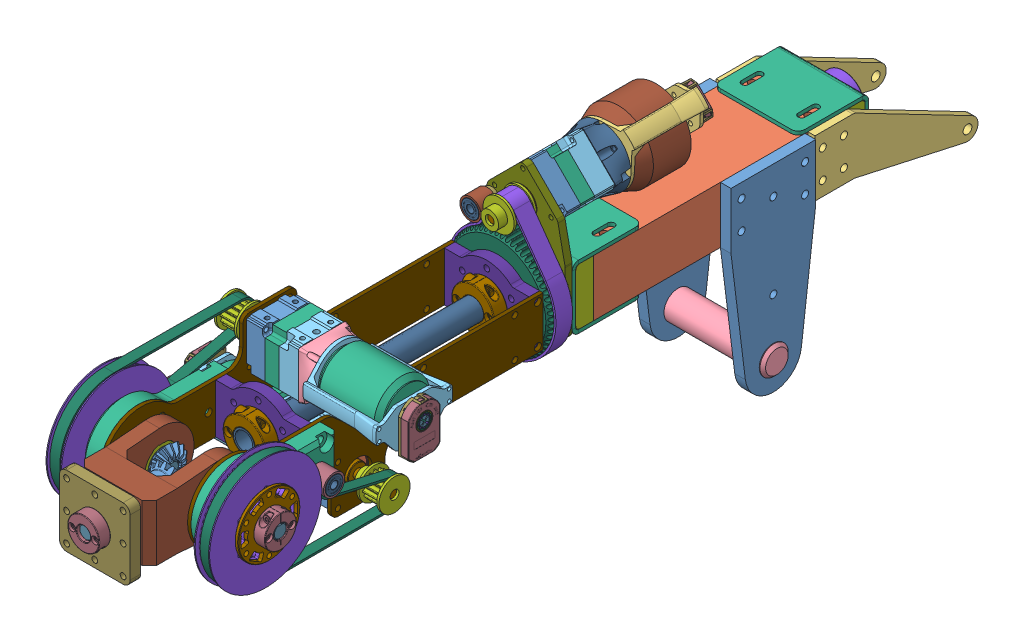
SolidWorks assembly Forearm, configuration Default. Lengths in mm. (continued)
Components (placement in the parent): (continued)
- 15Tpulley-4: 15Tpulley [Default] at (0 823.07 189.5517) x (-0.382318 -0.924031 0) z (-0.924031 0.382318 0) size (28 28 28)
- 15Tpulley-5: 15Tpulley [Default] at (-64.1092 796.898 367.2673) x (0 -1 0) z (0 0 1) size (28 28 28)
- 15Tpulley-6: 15Tpulley [Default] at (64.1092 726.052 367.2673) x (0 1 0) z (0 0 1) size (28 28 28)
- J4Belt^Forearm-1: J4Belt^Forearm [Default] at origin size (97.23 123.02 15) (virtual)
- TensionPillarJ4-1: TensionPillarJ4 [Default] at (30.7519 716.5034 107.0507) x (-0.923728 -0.383049 0) z (0.383049 -0.923728 0) size (19.05 19.38 19.05)
  - 98019A228_MIL SPEC. 300 SERIES SS FLAT WASHER-1: 98019A228_MIL SPEC. 300 SERIES SS FLAT WASHER [98019A228] at (17.4581 -74.6355 -111.1226) x (0.972939 0 -0.231063) z (0.231063 0 0.972939) size (9.53 0.71 9.53)
  - 60355K701_BALL BEARING-1: 60355K701_BALL BEARING [60355K701] at (17.4581 -77.1247 -111.1226) x (1 0 0) z (0 1 0) size (15.88 15.88 4.98)
  - Roller^TensionPillarJ4-1: Roller^TensionPillarJ4 [Default] at (-4.9135 -16.9545 2.0107) size (19.05 15 19.05) (virtual)
  - 60355K701_BALL BEARING-2: 60355K701_BALL BEARING [60355K701] at (17.4581 -87.6441 -111.1226) x (1 0 0) z (0 1 0) size (15.88 15.88 4.98)
  - 92510A483_ALUM UNTHRD SPACER-1: 92510A483_ALUM UNTHRD SPACER [92510A483] at (17.4581 -72.3368 -111.1226) x (1 0 0) z (0 1 0) size (15.88 15.88 3.17)
- TensionPillarJ56-1: TensionPillarJ56 [Default] at (15.1868 665.5152 480.9669) x (0 -0.383049 -0.923728) z (0 -0.923728 0.383049) size (19.05 17.8 19.05)
  - 98019A228_MIL SPEC. 300 SERIES SS FLAT WASHER-1: 98019A228_MIL SPEC. 300 SERIES SS FLAT WASHER [98019A228] at (17.4581 -74.6355 -111.1226) x (0.972939 0 -0.231063) z (0.231063 0 0.972939) size (9.53 0.71 9.53)
  - 60355K701_BALL BEARING-1: 60355K701_BALL BEARING [60355K701] at (17.4581 -77.1247 -111.1226) x (1 0 0) z (0 1 0) size (15.88 15.88 4.98)
  - Roller^TensionPillarJ56-1: Roller^TensionPillarJ56 [Default] at (-4.9135 -16.9545 2.0107) size (19.05 15 19.05) (virtual)
  - 60355K701_BALL BEARING-2: 60355K701_BALL BEARING [60355K701] at (17.4581 -87.6441 -111.1226) x (1 0 0) z (0 1 0) size (15.88 15.88 4.98)
  - 92510A398_ALUM UNTHRD SPACER-1: 92510A398_ALUM UNTHRD SPACER [92510A398] at (17.4581 -73.1305 -111.1226) x (1 0 0) z (0 1 0) size (12.7 12.7 1.59)
- J56Belt^Forearm-1: J56Belt^Forearm [Default] at origin size (9 97.23 176.76) (virtual)
- TensionPillarJ56-2: TensionPillarJ56 [Default] at (-15.1868 870.8093 395.8361) x (0 -0.383049 -0.923728) z (0 0.923728 -0.383049) size (19.05 17.8 19.05)
  - 98019A228_MIL SPEC. 300 SERIES SS FLAT WASHER-1: 98019A228_MIL SPEC. 300 SERIES SS FLAT WASHER [98019A228] at (17.4581 -74.6355 -111.1226) x (0.972939 0 -0.231063) z (0.231063 0 0.972939) size (9.53 0.71 9.53)
  - 60355K701_BALL BEARING-1: 60355K701_BALL BEARING [60355K701] at (17.4581 -77.1247 -111.1226) x (1 0 0) z (0 1 0) size (15.88 15.88 4.98)
  - Roller^TensionPillarJ56-1: Roller^TensionPillarJ56 [Default] at (-4.9135 -16.9545 2.0107) size (19.05 15 19.05) (virtual)
  - 60355K701_BALL BEARING-2: 60355K701_BALL BEARING [60355K701] at (17.4581 -87.6441 -111.1226) x (1 0 0) z (0 1 0) size (15.88 15.88 4.98)
  - 92510A398_ALUM UNTHRD SPACER-1: 92510A398_ALUM UNTHRD SPACER [92510A398] at (17.4581 -73.1305 -111.1226) x (1 0 0) z (0 1 0) size (12.7 12.7 1.59)
- J56Belt^Forearm-2: J56Belt^Forearm [Default] at (0 1522.95 0) x (-1 0 0) z (0 0 1) size (9 97.23 176.76) (virtual)
Mates (geometry in assembly coordinates):
- Concentric1: concentric anti-aligned: cylinder of SidePlate^Forearm-1 through (-47.625 634.475 0) axis (1 0 0) radius 12.7; circle of 6061K602_HARDENED PRECISION STEEL SHAFT-1
- Width1: width anti-aligned: plane of 6061K602_HARDENED PRECISION STEEL SHAFT-1 through (-50.8 634.475 0) normal (-1 0 0); plane of 6061K602_HARDENED PRECISION STEEL SHAFT-1 through (50.8 634.475 0) normal (1 0 0); plane of SidePlate^Forearm-2 through (47.625 634.475 0) normal (1 0 0); plane of SidePlate^Forearm-1 through (-47.625 634.475 0) normal (-1 0 0)
- Concentric2: concentric aligned: cylinder of 6384K367_BALL BEARING-1 through (0 761.475 160.274) axis (0 0 -1) radius 20.6375; cylinder of BearingHolder^Forearm-1 through (0 761.475 171.45) axis (0 0 -1) radius 20.6375
- Coincident2: coincident anti-aligned: plane of 6384K367_BALL BEARING-1 through (0 746.0646 171.45) normal (0 0 -1); plane of BearingHolder^Forearm-1 through (0 0 171.45) normal (0 0 1)
- Concentric3: concentric aligned: cylinder of 6384K367_BALL BEARING-2 through (0 761.475 -84.074) axis (0 0 1) radius 9.525; cylinder of 6435K160_ONE-PIECE CLAMP-ON SHAFT COLLAR-1 through (0 761.475 -111.0742) axis (0 0 1) radius 9.525
- Coincident3: coincident anti-aligned: plane of 6384K367_BALL BEARING-2 through (0 750.6038 -98.3742) normal (0 0 -1); plane of 6435K160_ONE-PIECE CLAMP-ON SHAFT COLLAR-1 through (0 761.475 -98.3742) normal (0 0 1)
- Concentric4: concentric anti-aligned: cylinder of 6384K367_BALL BEARING-1 through (0 761.475 160.274) axis (0 0 -1) radius 9.525; cylinder of 9677T100_CLAMP-ON SHAFT COLLAR WITH MOUNTING HOLES-1 through (0 761.475 210.2517) axis (0 0 1) radius 9.525
- Concentric5: concentric anti-aligned: cylinder of 89955K599_Tube^Forearm-1 through (0 761.475 455.5658) axis (0 0 -1) radius 9.525; cylinder of 5909K460_THRUST NEEDLE-ROLLER BEARING-1 through (0 761.475 187.5917) axis (0 0 1) radius 9.5504
- Coincident4: coincident anti-aligned: plane of ThrustBase^Forearm-1 through (0 761.475 187.5917) normal (0 0 1); plane of 5909K460_THRUST NEEDLE-ROLLER BEARING-1 through (0 761.475 187.5917) normal (0 0 -1)
- Concentric6: concentric anti-aligned: cylinder of 89955K599_Tube^Forearm-1 through (0 761.475 455.5658) axis (0 0 -1) radius 9.525; cylinder of 5909K330_THRUST NEEDLE-ROLLER BEARING-1 through (0 761.475 190.3889) axis (0 0 1) radius 9.5504
- Tangent1: tangent anti-aligned: plane of 5909K460_THRUST NEEDLE-ROLLER BEARING-1 through (0 761.475 188.4045) normal (0 0 1); cylinder of 5909K330_THRUST NEEDLE-ROLLER BEARING-1 through (-5.4469 747.7178 189.3967) axis (-0.368125 -0.929776 0) radius 0.9922
- Concentric7: concentric anti-aligned: cylinder of 89955K599_Tube^Forearm-1 through (0 761.475 455.5658) axis (0 0 -1) radius 9.525; cylinder of 5909K460_THRUST NEEDLE-ROLLER BEARING-2 through (0 761.475 190.3889) axis (0 0 1) radius 9.5504
- Tangent2: tangent anti-aligned: cylinder of 5909K330_THRUST NEEDLE-ROLLER BEARING-1 through (-1.8545 746.7954 189.3967) axis (-0.125333 -0.992115 0) radius 0.9922; plane of 5909K460_THRUST NEEDLE-ROLLER BEARING-2 through (0 761.475 190.3889) normal (0 0 -1)
- Concentric8: concentric anti-aligned: cylinder of 89955K599_Tube^Forearm-1 through (0 761.475 455.5658) axis (0 0 -1) radius 9.525; circle of J4Pulley-1
- Coincident6: coincident anti-aligned: plane of PulleySupportPlate^Forearm-1 through (0 0 194.3767) normal (0 0 1); plane of J4Pulley-1 through (0 761.475 194.3767) normal (0 0 -1)
- Parallel1: parallel anti-aligned: plane of 9677T100_CLAMP-ON SHAFT COLLAR WITH MOUNTING HOLES-1 through (0.0953 780.5248 210.2517) normal (-1 0 0)
- Coincident11: coincident anti-aligned: plane of 9677T100_CLAMP-ON SHAFT COLLAR WITH MOUNTING HOLES-1 through (0 761.475 210.2517) normal (0 0 -1); plane of WristHub^Forearm-1 through (-24.5934 788.4625 210.2517) normal (0 0 1)
- Concentric10: concentric aligned: cylinder of 89955K599_Tube^Forearm-1 through (0 761.475 455.5658) axis (0 0 -1) radius 9.525; cylinder of WristHub^Forearm-2 through (0 761.475 415.925) axis (0 0 -1) radius 9.525
- Distance2: distance = 406.4 mm: plane of assembly through (0 0 0) normal (0 0 1); plane of assembly; plane of WristHub^Forearm-2 through (-24.5934 788.4625 406.4) normal (0 0 -1)
- Concentric11: concentric anti-aligned: cylinder of 89955K599_Tube^Forearm-1 through (0 761.475 455.5658) axis (0 0 -1) radius 7.9375; cylinder of 9677T100_CLAMP-ON SHAFT COLLAR WITH MOUNTING HOLES-2 through (0 761.475 415.925) axis (0 0 1) radius 9.525
- Coincident13: coincident anti-aligned: plane of WristHub^Forearm-2 through (-24.5934 788.4625 415.925) normal (0 0 1); plane of 9677T100_CLAMP-ON SHAFT COLLAR WITH MOUNTING HOLES-2 through (0 761.475 415.925) normal (0 0 -1)
- Concentric12: concentric anti-aligned: cylinder of WristSidePlate^Forearm-1 through (-41.275 761.475 482.6) axis (1 0 0) radius 14.2875; cylinder of 6843K130_MTL MITER GEAR--20 DEG PRESSURE ANGLE-1 through (31.0355 761.475 482.6) axis (-1 0 0) radius 6.3563
- Concentric13: concentric anti-aligned: cylinder of 89955K599_Tube^Forearm-1 through (0 761.475 455.5658) axis (0 0 -1) radius 7.9375; cylinder of 6843K130_MTL MITER GEAR--20 DEG PRESSURE ANGLE-3 through (0 761.475 451.5645) axis (0 0 1) radius 6.3563
- Distance3: distance = 31.75 mm: cylinder of 6843K130_MTL MITER GEAR--20 DEG PRESSURE ANGLE-3 through (0 761.475 451.5645) axis (0 0 1) radius 6.3563; plane of 6843K130_MTL MITER GEAR--20 DEG PRESSURE ANGLE-1 through (-31.75 761.253 469.9019) normal (-1 0 0)
- Distance4: distance = 31.75 mm: plane of 6843K130_MTL MITER GEAR--20 DEG PRESSURE ANGLE-3 through (-12.6981 761.253 514.35) normal (0 0 1); cylinder of 6843K130_MTL MITER GEAR--20 DEG PRESSURE ANGLE-1 through (31.0355 761.475 482.6) axis (-1 0 0) radius 6.3563
- Concentric14: concentric anti-aligned: cylinder of WristSidePlate^Forearm-1 through (-41.275 761.475 482.6) axis (1 0 0) radius 14.2875; cylinder of 6384K361_BALL BEARING-1-1 through (-46.101 761.475 482.6) axis (-1 0 0) radius 14.2875
- Coincident14: coincident anti-aligned: plane of WristSidePlate^Forearm-1 through (-38.1 0 0) normal (1 0 0); plane of 6384K361_BALL BEARING-1-1 through (-38.1 772.1938 482.6) normal (-1 0 0)
- Concentric15: concentric aligned: cylinder of 6843K130_MTL MITER GEAR--20 DEG PRESSURE ANGLE-1 through (31.0355 761.475 482.6) axis (-1 0 0) radius 6.3563; cylinder of 5909K440_THRUST NEEDLE-ROLLER BEARING-1 through (-33.7344 761.475 482.6) axis (-1 0 0) radius 6.3754
- Concentric16: concentric anti-aligned: cylinder of 6843K130_MTL MITER GEAR--20 DEG PRESSURE ANGLE-1 through (31.0355 761.475 482.6) axis (-1 0 0) radius 6.3563; cylinder of 5909K310_THRUST NEEDLE-ROLLER BEARING-1 through (-31.75 761.475 482.6) axis (1 0 0) radius 6.3754
- Tangent6: tangent anti-aligned: plane of 6843K130_MTL MITER GEAR--20 DEG PRESSURE ANGLE-1 through (-31.75 761.253 469.9019) normal (-1 0 0); cylinder of 5909K310_THRUST NEEDLE-ROLLER BEARING-1 through (-32.7422 750.594 485.3554) axis (0 -0.9694 0.245485) radius 0.9922
- Tangent7: tangent anti-aligned: plane of 5909K440_THRUST NEEDLE-ROLLER BEARING-1 through (-33.7344 761.475 482.6) normal (1 0 0); cylinder of 5909K310_THRUST NEEDLE-ROLLER BEARING-1 through (-32.7422 750.594 485.3554) axis (0 -0.9694 0.245485) radius 0.9922
- Concentric17: concentric aligned: cylinder of 6384K361_BALL BEARING-1-2 through (-49.149 761.475 482.6) axis (1 0 0) radius 14.2875; cylinder of SidePrintedSupport^Forearm-1 through (-57.15 761.475 482.6) axis (1 0 0) radius 14.2875
- Coincident16: coincident anti-aligned: plane of SidePrintedSupport^Forearm-1 through (-57.15 0 0) normal (-1 0 0); plane of 6384K361_BALL BEARING-1-2 through (-57.15 750.7562 482.6) normal (1 0 0)
- Concentric18: concentric anti-aligned: cylinder of 6843K130_MTL MITER GEAR--20 DEG PRESSURE ANGLE-1 through (31.0355 761.475 482.6) axis (-1 0 0) radius 12.7; cylinder of 6391K281_OIL-EMBEDDED SLEEVE BEARING-1 through (-32.2445 761.475 482.6) axis (1 0 0) radius 12.7
- Concentric20: concentric anti-aligned: cylinder of 6384K361_BALL BEARING-1-2 through (-49.149 761.475 482.6) axis (1 0 0) radius 6.35; cylinder of PulleyHubbed-1/1_2_ID_1_8_Keyway_Aluminum_VersaHub_217-2590 v1-1 through (-64.0842 761.475 482.6) axis (-1 0 0) radius 6.3627
- Coincident18: coincident anti-aligned: plane of PulleyHubbed-1/1_2_ID_1_8_Keyway_Aluminum_VersaHub_217-2590 v1-1 through (-64.0842 761.475 482.6) normal (1 0 0); plane of SidePulleySpacer^Forearm-1 through (-64.0842 761.475 482.6) normal (-1 0 0)
- Concentric21: concentric anti-aligned: cylinder of WristBase^Forearm-3 through (0 761.475 546.1) axis (0 0 -1) radius 14.2875; cylinder of 6384K361_BALL BEARING-1-5 through (0 761.475 528.701) axis (0 0 1) radius 14.2875
- Coincident19: coincident anti-aligned: plane of WristBase^Forearm-3 through (0 0 520.7) normal (0 0 -1); plane of 6384K361_BALL BEARING-1-5 through (0 772.1938 520.7) normal (0 0 1)
- Concentric22: concentric anti-aligned: cylinder of WristBase^Forearm-3 through (0 761.475 546.1) axis (0 0 -1) radius 14.2875; cylinder of MiterSpacer^Forearm-3 through (0 761.475 472.2459) axis (0 0 1) radius 9.3726
- Coincident21: coincident anti-aligned: plane of 6384K361_BALL BEARING-1-5 through (0 775.2862 519.176) normal (0 0 -1); plane of MiterSpacer^Forearm-3 through (0 761.475 519.176) normal (0 0 1)
- Concentric23: concentric anti-aligned: cylinder of WristBase^Forearm-3 through (0 761.475 546.1) axis (0 0 -1) radius 14.2875; cylinder of 5909K440_THRUST NEEDLE-ROLLER BEARING-3 through (0 761.475 516.3344) axis (0 0 1) radius 6.3754
- Coincident22: coincident anti-aligned: plane of MiterSpacer^Forearm-3 through (0 761.475 517.1472) normal (0 0 -1); plane of 5909K440_THRUST NEEDLE-ROLLER BEARING-3 through (0 761.475 517.1472) normal (0 0 1)
- Concentric24: concentric anti-aligned: cylinder of WristBase^Forearm-3 through (0 761.475 546.1) axis (0 0 -1) radius 14.2875; cylinder of 5909K310_THRUST NEEDLE-ROLLER BEARING-3 through (0 761.475 516.3344) axis (0 0 1) radius 6.3754
- Tangent8: tangent anti-aligned: plane of 6843K130_MTL MITER GEAR--20 DEG PRESSURE ANGLE-3 through (-12.6981 761.253 514.35) normal (0 0 1); cylinder of 5909K310_THRUST NEEDLE-ROLLER BEARING-3 through (-8.8576 768.3692 515.3422) axis (-0.789141 0.614213 0) radius 0.9922
- Concentric25: concentric aligned: cylinder of WristBase^Forearm-3 through (0 761.475 546.1) axis (0 0 -1) radius 14.2875; cylinder of 6384K361_BALL BEARING-1-6 through (0 761.475 538.099) axis (0 0 -1) radius 14.2875
- Coincident24: coincident anti-aligned: plane of WristBase^Forearm-3 through (0 0 546.1) normal (0 0 1); plane of 6384K361_BALL BEARING-1-6 through (0 750.7562 546.1) normal (0 0 -1)
- Concentric26: concentric anti-aligned: cylinder of 6384K361_BALL BEARING-1-6 through (0 761.475 538.099) axis (0 0 -1) radius 6.35; cylinder of MiterSpacer^Forearm-4 through (0 761.475 502.7227) axis (0 0 1) radius 9.3726
- Coincident25: coincident anti-aligned: plane of 6384K361_BALL BEARING-1-6 through (0 747.6637 547.624) normal (0 0 1); plane of MiterSpacer^Forearm-4 through (0 761.475 547.624) normal (0 0 -1)
- Concentric27: concentric anti-aligned: cylinder of 6384K361_BALL BEARING-1-6 through (0 761.475 538.099) axis (0 0 -1) radius 6.35; cylinder of 5909K440_THRUST NEEDLE-ROLLER BEARING-4 through (0 761.475 549.6528) axis (0 0 1) radius 6.3754
- Coincident26: coincident anti-aligned: plane of MiterSpacer^Forearm-4 through (0 761.475 549.6528) normal (0 0 1); plane of 5909K440_THRUST NEEDLE-ROLLER BEARING-4 through (0 761.475 549.6528) normal (0 0 -1)
- Concentric28: concentric anti-aligned: cylinder of 6384K361_BALL BEARING-1-6 through (0 761.475 538.099) axis (0 0 -1) radius 6.35; cylinder of 5909K310_THRUST NEEDLE-ROLLER BEARING-4 through (0 761.475 552.45) axis (0 0 1) radius 6.3754
- Tangent9: tangent anti-aligned: plane of 5909K440_THRUST NEEDLE-ROLLER BEARING-4 through (0 761.475 550.4656) normal (0 0 1); cylinder of 5909K310_THRUST NEEDLE-ROLLER BEARING-4 through (-6.1392 752.0783 551.4578) axis (-0.546948 -0.837166 0) radius 0.9922
- Tangent10: tangent anti-aligned: plane of 5909K440_THRUST NEEDLE-ROLLER BEARING-5 through (0 761.475 552.45) normal (0 0 -1); cylinder of 5909K310_THRUST NEEDLE-ROLLER BEARING-4 through (-2.7554 750.594 551.4578) axis (-0.245485 -0.9694 0) radius 0.9922
- Concentric29: concentric anti-aligned: cylinder of 6384K361_BALL BEARING-1-6 through (0 761.475 538.099) axis (0 0 -1) radius 6.35; cylinder of 5909K440_THRUST NEEDLE-ROLLER BEARING-5 through (0 761.475 552.45) axis (0 0 1) radius 6.3754
- Concentric39: concentric anti-aligned: cylinder of HandPlate^Forearm-1 through (0 761.475 562.7878) axis (0 0 -1) radius 6.35; cylinder of 9677T210_CLAMP-ON SHAFT COLLAR WITH MOUNTING HOLES-1 through (0 761.475 562.7878) axis (0 0 1) radius 6.35
- Coincident29: coincident anti-aligned: plane of HandPlate^Forearm-1 through (0 0 562.7878) normal (0 0 1); plane of 9677T210_CLAMP-ON SHAFT COLLAR WITH MOUNTING HOLES-1 through (0 761.475 562.7878) normal (0 0 -1)
- Concentric40: concentric aligned: cylinder of PulleyHubbed-1/1_2_ID_1_8_Keyway_Aluminum_VersaHub_217-2590 v1-1 through (-64.0842 761.475 482.6) axis (-1 0 0) radius 6.3627; cylinder of 9677T210_CLAMP-ON SHAFT COLLAR WITH MOUNTING HOLES-2 through (-76.7842 761.475 482.6) axis (-1 0 0) radius 6.35
- Coincident30: coincident anti-aligned: plane of PulleyHubbed-1/1_2_ID_1_8_Keyway_Aluminum_VersaHub_217-2590 v1-1 through (-76.7842 729.9282 482.6) normal (-1 0 0); plane of 9677T210_CLAMP-ON SHAFT COLLAR WITH MOUNTING HOLES-2 through (-76.7842 761.475 482.6) normal (1 0 0)
- Concentric41: concentric anti-aligned: cylinder of 6384K361_BALL BEARING-1-1 through (-46.101 761.475 482.6) axis (-1 0 0) radius 6.35; cylinder of 8488T310_FULLY KEYED PRECISION DRIVE SHAFT W CERT-1 through (-86.6172 761.475 482.6) axis (1 0 0) radius 6.35
- Width2: width anti-aligned: plane of 8488T310_FULLY KEYED PRECISION DRIVE SHAFT W CERT-1 through (-86.6172 761.475 482.6) normal (-1 0 0); plane of 6843K130_MTL MITER GEAR--20 DEG PRESSURE ANGLE-1 through (-10.4172 761.475 482.6) normal (1 0 0); plane of 8488T310_FULLY KEYED PRECISION DRIVE SHAFT W CERT-1 through (-9.9314 761.3639 476.2446) normal (1 0 0); plane of 9677T210_CLAMP-ON SHAFT COLLAR WITH MOUNTING HOLES-2 through (-87.1029 761.475 482.6) normal (-1 0 0)
- Coincident32: coincident anti-aligned: circle of 6843K130_MTL MITER GEAR--20 DEG PRESSURE ANGLE-1; plane of 6391K281_OIL-EMBEDDED SLEEVE BEARING-1 through (-19.5445 761.475 482.6) normal (1 0 0)
- Concentric42: concentric anti-aligned: cylinder of 9677T210_CLAMP-ON SHAFT COLLAR WITH MOUNTING HOLES-1 through (0 761.475 562.7878) axis (0 0 1) radius 6.35; cylinder of 8488T310_FULLY KEYED PRECISION DRIVE SHAFT W CERT-3 through (0 761.475 570.919) axis (0 0 -1) radius 6.35
- Width3: width aligned: plane of 8488T310_FULLY KEYED PRECISION DRIVE SHAFT W CERT-3 through (0 761.475 570.919) normal (0 0 1); plane of 8488T310_FULLY KEYED PRECISION DRIVE SHAFT W CERT-3 through (0 761.475 494.719) normal (0 0 -1); plane of 9677T210_CLAMP-ON SHAFT COLLAR WITH MOUNTING HOLES-1 through (0 761.475 573.1065) normal (0 0 1); plane of 6843K130_MTL MITER GEAR--20 DEG PRESSURE ANGLE-3 through (-6.3554 761.3639 492.5314) normal (0 0 -1)
- Concentric44: concentric aligned: cylinder of J4MotorPlate^Forearm-1 through (0 823.07 177.8) axis (0 0 -1) radius 12.7; cylinder of Keda9to1-1/VersaPlanetary_CIM_Motor_Output_Shaft_Kit_217-2893-1 through (0 823.07 248.5932) axis (0 0 -1) radius 3.975
- Concentric45: concentric aligned: cylinder of J4MotorPlate^Forearm-1 through (0 848.47 177.8) axis (0 0 -1) radius 1.9844; cylinder of Keda9to1-1/VersaPlanetary_v2_Single_Stage_10_1_with_BAG.STEP-1/217-2625-026 Rev1.STEP-1 through (0 848.47 154.825) axis (0 0 -1) radius 2.0193
- Coincident33: coincident anti-aligned: plane of J4MotorPlate^Forearm-1 through (0 0 171.45) normal (0 0 -1); plane of Keda9to1-1/VersaPlanetary_v2_Single_Stage_10_1_with_BAG.STEP-1/217-2625-026 Rev1.STEP-1 through (-31.4309 823.07 171.45) normal (0 0 1)
- Concentric46: concentric anti-aligned: cylinder of WristSidePlate^Forearm-1 through (-41.275 796.898 367.2673) axis (1 0 0) radius 12.7; cylinder of PropDrive10to1-2/VersaPlanetary_CIM_Motor_Output_Shaft_Kit_217-2893-1 through (-36.6752 796.898 367.2673) axis (-1 0 0) radius 8.5
- Coincident34: coincident anti-aligned: plane of WristSidePlate^Forearm-1 through (-38.1 0 0) normal (1 0 0); plane of PropDrive10to1-2/VersaPlanetary_v2_Single_Stage_10_1_with_BAG.STEP-1/217-2625-026 Rev1.STEP-1 through (-38.1 774.673 389.4923) normal (-1 0 0)
- Parallel3: parallel anti-aligned: plane of PropDrive10to1-2 through (-21.475 819.123 367.2673) normal (0 -1 0)
- Concentric49: concentric anti-aligned: cylinder of WristHub^Forearm-1 through (25.4 778.9375 205.4892) axis (1 0 0) radius 2.6035; cylinder of WristSidePlate^Forearm-3 through (41.275 778.9375 205.4892) axis (-1 0 0) radius 3.175
- Coincident36: coincident anti-aligned: plane of WristHub^Forearm-1 through (38.1 783.7 210.2517) normal (1 0 0); plane of WristSidePlate^Forearm-3 through (38.1 1522.95 0) normal (-1 0 0)
- Concentric50: concentric anti-aligned: cylinder of WristHub^Forearm-1 through (25.4 744.0125 205.4892) axis (1 0 0) radius 2.6035; cylinder of WristSidePlate^Forearm-3 through (41.275 744.0125 205.4892) axis (-1 0 0) radius 3.175
- Concentric51: concentric anti-aligned: cylinder of WristSidePlate^Forearm-3 through (41.275 726.052 367.2673) axis (-1 0 0) radius 12.7; cylinder of PropDrive10to1-4/VersaPlanetary_CIM_Motor_Output_Shaft_Kit_217-2893-1 through (36.6752 726.052 367.2673) axis (1 0 0) radius 8.5
- Coincident37: coincident anti-aligned: plane of WristSidePlate^Forearm-3 through (38.1 1522.95 0) normal (-1 0 0); plane of PropDrive10to1-4/VersaPlanetary_v2_Single_Stage_10_1_with_BAG.STEP-1/217-2625-026 Rev1.STEP-1 through (38.1 748.277 389.4923) normal (1 0 0)
- Parallel4: parallel anti-aligned: plane of PropDrive10to1-4/380kvMotorEncoded-1/PROPDRIVE v2 5060 380KV Brushless Outrunner Motor-1 through (-26.5443 726.052 367.2673) normal (0 -1 0)
- Concentric52: concentric aligned: cylinder of Keda9to1-1/VersaPlanetary_CIM_Motor_Output_Shaft_Kit_217-2893-1 through (0 823.07 248.5932) axis (0 0 -1) radius 3.975; cylinder of 15Tpulley-4 through (0 823.07 197.5517) axis (0 0 -1) radius 4
- Distance5: distance = 3.175 mm anti-aligned: plane of 15Tpulley-4 through (0 823.07 197.5517) normal (0 0 -1); plane of J4Pulley-1 through (0 761.475 200.7267) normal (0 0 1)
- Concentric53: concentric anti-aligned: cylinder of PropDrive10to1-2/VersaPlanetary_CIM_Motor_Output_Shaft_Kit_217-2893-1 through (-115.2432 796.898 367.2673) axis (1 0 0) radius 3.975; cylinder of 15Tpulley-5 through (-56.1092 796.898 367.2673) axis (-1 0 0) radius 4
- Coincident40: coincident aligned: plane of PulleyHubbed-1/60t_x_18mm_Wide_VersaPulley_Kit_HTD_5mm_VersaKeys_217-3200 v2-1/60t_x_18mm_Wide_VersaPulley_Kit_HTD_5mm_VersaKeys_217-3200 v2.step-1/217-3200-001 Rev3.step-1 through (-72.1092 761.475 482.6) normal (1 0 0); plane of 15Tpulley-5 through (-72.1092 796.898 367.2673) normal (1 0 0)
- Concentric54: concentric anti-aligned: cylinder of PropDrive10to1-4/VersaPlanetary_CIM_Motor_Output_Shaft_Kit_217-2893-1 through (115.2432 726.052 367.2673) axis (-1 0 0) radius 3.975; cylinder of 15Tpulley-6 through (56.1092 726.052 367.2673) axis (1 0 0) radius 4
- Coincident42: coincident aligned: plane of PulleyHubbed-2/60t_x_18mm_Wide_VersaPulley_Kit_HTD_5mm_VersaKeys_217-3200 v2-1/60t_x_18mm_Wide_VersaPulley_Kit_HTD_5mm_VersaKeys_217-3200 v2.step-1/217-3200-001 Rev3.step-1 through (72.1092 761.475 482.6) normal (-1 0 0); plane of 15Tpulley-6 through (72.1092 726.052 367.2673) normal (-1 0 0)
- Concentric55: concentric aligned: cylinder of J4MotorPlate^Forearm-1 through (-27.94 812.4631 162.4697) axis (0 0 1) radius 3.175; cylinder of TensionPillarJ4-1/92510A483_ALUM UNTHRD SPACER-1 through (-27.94 812.4631 177.8) axis (0 0 1) radius 3.2004
- Coincident44: coincident anti-aligned: plane of J4MotorPlate^Forearm-1 through (0 0 177.8) normal (0 0 1); plane of TensionPillarJ4-1/92510A483_ALUM UNTHRD SPACER-1 through (-27.94 812.4631 177.8) normal (0 0 -1)
- Concentric57: concentric anti-aligned: cylinder of SidePrintedSupport^Forearm-1 through (-57.15 761.475 422.275) axis (1 0 0) radius 3.175; cylinder of TensionPillarJ56-1/92510A398_ALUM UNTHRD SPACER-1 through (-57.15 761.475 422.275) axis (-1 0 0) radius 3.2004
- Coincident46: coincident anti-aligned: plane of SidePrintedSupport^Forearm-1 through (-57.15 0 0) normal (-1 0 0); plane of TensionPillarJ56-1/92510A398_ALUM UNTHRD SPACER-1 through (-57.15 761.475 422.275) normal (1 0 0)
